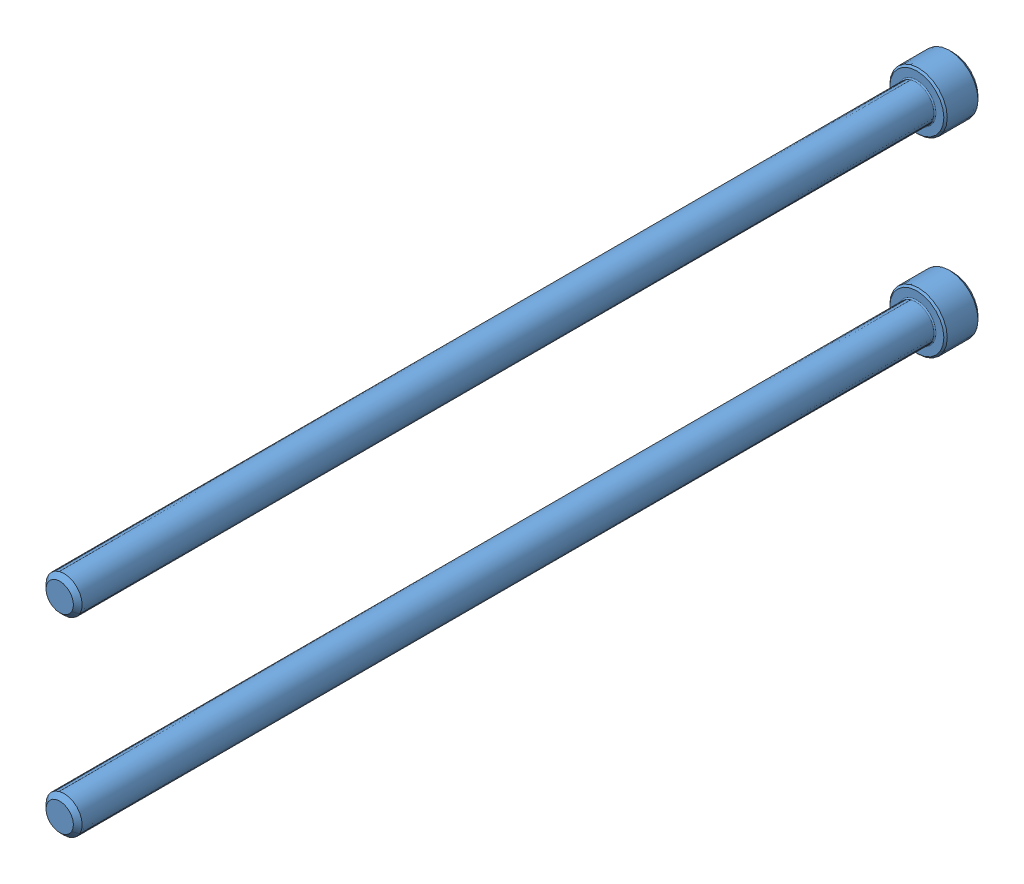
SolidWorks assembly WCP - GreyT Elevator (Cascade, 2 Stage) (1).step, configuration Default. Lengths in mm.
Overall size (10.46 35.86 119.13).
407 component instances, 66 part files, 0 mates.
Components (placement in the parent):
- WCP-0323 - Elevator Clamping Block.step-1: WCP-0323 - Elevator Clamping Block.step [Default] at (152.3365 1149.35 -25.4) x (0 0 1) z (-1 0 0) size (29.22 25.41 49.35) (hidden)
  - WCP-0323-001 Rev2.step-1: WCP-0323-001 Rev2.step [Default] at origin size (20.38 25.41 40.49)
  - WCP-0498 Rev1.step-1: WCP-0498 Rev1.step [Default] at (2.254 0 6.7) x (0 0.307359 0.951594) z (-1 0 0) size (12 12 4)
  - WCP-0212_0_250_radial_bearing.step-1: WCP-0212_0_250_radial_bearing.step [Default] at (-9.525 0 15.4781) size (19.05 19.05 7.14)
  - WCP-0473 Rev1.step-1: WCP-0473 Rev1.step [Default] at (-9.525 0 10.4394) x (-0.082744 -0.996571 0) z (-0.996571 0.082744 0) size (9.53 20.65 9.53)
  - #8-32 x .25L BHCS.step-1: #8-32 x .25L BHCS.step [Default] at (6.7178 0 6.7) x (0 -0.337236 -0.94142) z (1 0 0) size (10.28 8 12.02)
- WCP-0323 - Elevator Clamping Block-1.step-1: WCP-0323 - Elevator Clamping Block-1.step [Default] at (152.3365 1149.35 25.4) x (0 0 -1) z (-1 0 0) size (29.22 25.41 49.35) (hidden)
  - WCP-0323-001 Rev2.step-1: WCP-0323-001 Rev2.step [Default] at origin size (20.38 25.41 40.49)
  - WCP-0498 Rev1.step-1: WCP-0498 Rev1.step [Default] at (2.254 0 6.7) x (0 0.307359 0.951594) z (-1 0 0) size (12 12 4)
  - WCP-0212_0_250_radial_bearing.step-1: WCP-0212_0_250_radial_bearing.step [Default] at (-9.525 0 15.4781) size (19.05 19.05 7.14)
  - WCP-0473 Rev1.step-1: WCP-0473 Rev1.step [Default] at (-9.525 0 10.4394) x (-0.082744 -0.996571 0) z (-0.996571 0.082744 0) size (9.53 20.65 9.53)
  - #8-32 x .25L BHCS.step-1: #8-32 x .25L BHCS.step [Default] at (6.7178 0 6.7) x (0 -0.337236 -0.94142) z (1 0 0) size (10.28 8 12.02)
- WCP-0323 - Elevator Clamping Block-2.step-1: WCP-0323 - Elevator Clamping Block-2.step [Default] at (139.7635 57.15 25.4) x (0 0 -1) z (1 0 0) size (29.22 25.41 49.35) (hidden)
  - WCP-0323-001 Rev2.step-1: WCP-0323-001 Rev2.step [Default] at origin size (20.38 25.41 40.49)
  - WCP-0498 Rev1.step-1: WCP-0498 Rev1.step [Default] at (2.254 0 6.7) x (0 0.307359 0.951594) z (-1 0 0) size (12 12 4)
  - WCP-0212_0_250_radial_bearing.step-1: WCP-0212_0_250_radial_bearing.step [Default] at (-9.525 0 15.4781) size (19.05 19.05 7.14)
  - WCP-0473 Rev1.step-1: WCP-0473 Rev1.step [Default] at (-9.525 0 10.4394) x (-0.082744 -0.996571 0) z (-0.996571 0.082744 0) size (9.53 20.65 9.53)
  - #8-32 x .25L BHCS.step-1: #8-32 x .25L BHCS.step [Default] at (6.7178 0 6.7) x (0 -0.337236 -0.94142) z (1 0 0) size (10.28 8 12.02)
- WCP-0323 - Elevator Clamping Block-3.step-1: WCP-0323 - Elevator Clamping Block-3.step [Default] at (139.7635 57.15 -25.4) x (0 0 1) z (1 0 0) size (29.22 25.41 49.35) (hidden)
  - WCP-0323-001 Rev2.step-1: WCP-0323-001 Rev2.step [Default] at origin size (20.38 25.41 40.49)
  - WCP-0498 Rev1.step-1: WCP-0498 Rev1.step [Default] at (2.254 0 6.7) x (0 0.307359 0.951594) z (-1 0 0) size (12 12 4)
  - WCP-0212_0_250_radial_bearing.step-1: WCP-0212_0_250_radial_bearing.step [Default] at (-9.525 0 15.4781) size (19.05 19.05 7.14)
  - WCP-0473 Rev1.step-1: WCP-0473 Rev1.step [Default] at (-9.525 0 10.4394) x (-0.082744 -0.996571 0) z (-0.996571 0.082744 0) size (9.53 20.65 9.53)
  - #8-32 x .25L BHCS.step-1: #8-32 x .25L BHCS.step [Default] at (6.7178 0 6.7) x (0 -0.337236 -0.94142) z (1 0 0) size (10.28 8 12.02)
- WCP-0323 - Elevator Clamping Block-4.step-1: WCP-0323 - Elevator Clamping Block-4.step [Default] at (101.6635 82.55 25.4) x (0 0 -1) z (1 0 0) size (29.22 25.41 49.35) (hidden)
  - WCP-0323-001 Rev2.step-1: WCP-0323-001 Rev2.step [Default] at origin size (20.38 25.41 40.49)
  - WCP-0498 Rev1.step-1: WCP-0498 Rev1.step [Default] at (2.254 0 6.7) x (0 0.307359 0.951594) z (-1 0 0) size (12 12 4)
  - WCP-0212_0_250_radial_bearing.step-1: WCP-0212_0_250_radial_bearing.step [Default] at (-9.525 0 15.4781) size (19.05 19.05 7.14)
  - WCP-0473 Rev1.step-1: WCP-0473 Rev1.step [Default] at (-9.525 0 10.4394) x (-0.082744 -0.996571 0) z (-0.996571 0.082744 0) size (9.53 20.65 9.53)
  - #8-32 x .25L BHCS.step-1: #8-32 x .25L BHCS.step [Default] at (6.7178 0 6.7) x (0 -0.337236 -0.94142) z (1 0 0) size (10.28 8 12.02)
- WCP-0323 - Elevator Clamping Block-5.step-1: WCP-0323 - Elevator Clamping Block-5.step [Default] at (101.6635 82.55 -25.4) x (0 0 1) z (1 0 0) size (29.22 25.41 49.35) (hidden)
  - WCP-0323-001 Rev2.step-1: WCP-0323-001 Rev2.step [Default] at origin size (20.38 25.41 40.49)
  - WCP-0498 Rev1.step-1: WCP-0498 Rev1.step [Default] at (2.254 0 6.7) x (0 0.307359 0.951594) z (-1 0 0) size (12 12 4)
  - WCP-0212_0_250_radial_bearing.step-1: WCP-0212_0_250_radial_bearing.step [Default] at (-9.525 0 15.4781) size (19.05 19.05 7.14)
  - WCP-0473 Rev1.step-1: WCP-0473 Rev1.step [Default] at (-9.525 0 10.4394) x (-0.082744 -0.996571 0) z (-0.996571 0.082744 0) size (9.53 20.65 9.53)
  - #8-32 x .25L BHCS.step-1: #8-32 x .25L BHCS.step [Default] at (6.7178 0 6.7) x (0 -0.337236 -0.94142) z (1 0 0) size (10.28 8 12.02)
- WCP-0323 - Elevator Clamping Block-6.step-1: WCP-0323 - Elevator Clamping Block-6.step [Default] at (101.6635 222.25 25.4) x (0 0 -1) z (1 0 0) size (29.22 25.41 49.35) (hidden)
  - WCP-0323-001 Rev2.step-1: WCP-0323-001 Rev2.step [Default] at origin size (20.38 25.41 40.49)
  - WCP-0498 Rev1.step-1: WCP-0498 Rev1.step [Default] at (2.254 0 6.7) x (0 0.307359 0.951594) z (-1 0 0) size (12 12 4)
  - WCP-0212_0_250_radial_bearing.step-1: WCP-0212_0_250_radial_bearing.step [Default] at (-9.525 0 15.4781) size (19.05 19.05 7.14)
  - WCP-0473 Rev1.step-1: WCP-0473 Rev1.step [Default] at (-9.525 0 10.4394) x (-0.082744 -0.996571 0) z (-0.996571 0.082744 0) size (9.53 20.65 9.53)
  - #8-32 x .25L BHCS.step-1: #8-32 x .25L BHCS.step [Default] at (6.7178 0 6.7) x (0 -0.337236 -0.94142) z (1 0 0) size (10.28 8 12.02)
- WCP-0323 - Elevator Clamping Block-7.step-1: WCP-0323 - Elevator Clamping Block-7.step [Default] at (101.6635 222.25 -25.4) x (0 0 1) z (1 0 0) size (29.22 25.41 49.35) (hidden)
  - WCP-0323-001 Rev2.step-1: WCP-0323-001 Rev2.step [Default] at origin size (20.38 25.41 40.49)
  - WCP-0498 Rev1.step-1: WCP-0498 Rev1.step [Default] at (2.254 0 6.7) x (0 0.307359 0.951594) z (-1 0 0) size (12 12 4)
  - WCP-0212_0_250_radial_bearing.step-1: WCP-0212_0_250_radial_bearing.step [Default] at (-9.525 0 15.4781) size (19.05 19.05 7.14)
  - WCP-0473 Rev1.step-1: WCP-0473 Rev1.step [Default] at (-9.525 0 10.4394) x (-0.082744 -0.996571 0) z (-0.996571 0.082744 0) size (9.53 20.65 9.53)
  - #8-32 x .25L BHCS.step-1: #8-32 x .25L BHCS.step [Default] at (6.7178 0 6.7) x (0 -0.337236 -0.94142) z (1 0 0) size (10.28 8 12.02)
- WCP-0248 Rev1 - #35 Chain Turnbuckle.step-1: WCP-0248 Rev1 - #35 Chain Turnbuckle.step [Default] at (88.9 1124.7437 -66.675) x (0 -1 0) z (0 0 1) size (55.56 15.05 15.04) (hidden)
  - WCP-0247-001 Rev1.step-1: WCP-0247-001 Rev1.step [Default] at origin size (30.16 9.53 11)
  - NFS-0040_#10-32_jam_nut_left_hand_99961A520.step-1: NFS-0040_#10-32_jam_nut_left_hand_99961A520.step [Default] at (-16.6687 0 0) x (0 0.5 -0.866025) z (0 0.866025 0.5) size (11.01 3.2 11.02)
  - NFS-0037_#10-32_jam_nut_90480A195.step-1: NFS-0037_#10-32_jam_nut_90480A195.step [Default] at (16.6687 0 0) x (0 0.5 0.866025) z (0 -0.866025 0.5) size (11.01 3.2 11.02)
  - WCP-0248-001 Rev1.step-1: WCP-0248-001 Rev1.step [Default] at (23.8125 0 0) x (0 0 1) z (0 1 0) size (9 25.4 9)
  - WCP-0248-002 Rev1.step-1: WCP-0248-002 Rev1.step [Default] at (-23.8125 0 0) x (0 0 -1) z (0 1 0) size (9 25.4 9)
- WCP-0247 Rev1 - #25 Chain Turnbuckle.step-1: WCP-0247 Rev1 - #25 Chain Turnbuckle.step [Default] at (-47.6339 1117.6 -50.8) x (0 1 0) z (-1 0 0) size (50.8 15.05 15.04) (hidden)
  - WCP-0247-001 Rev1.step-1: WCP-0247-001 Rev1.step [Default] at origin size (30.16 9.53 11)
  - NFS-0040_#10-32_jam_nut_left_hand_99961A520.step-1: NFS-0040_#10-32_jam_nut_left_hand_99961A520.step [Default] at (-16.6687 0 0) x (0 0.5 -0.866025) z (0 0.866025 0.5) size (11.01 3.2 11.02)
  - NFS-0037_#10-32_jam_nut_90480A195.step-1: NFS-0037_#10-32_jam_nut_90480A195.step [Default] at (16.6687 0 0) x (0 0.5 0.866025) z (0 -0.866025 0.5) size (11.01 3.2 11.02)
  - WCP-0247-002 Rev2.step-1: WCP-0247-002 Rev2.step [Default] at (22.225 0 0) x (0 0 1) z (0 1 0) size (9 23.02 5.21)
  - WCP-0247-003 Rev2.step-1: WCP-0247-003 Rev2.step [Default] at (-22.225 0 0) x (0 0 -1) z (0 1 0) size (9 23.02 5.21)
- WCP-0323 - Elevator Clamping Block-8.step-1: WCP-0323 - Elevator Clamping Block-8.step [Default] at (-152.3365 1149.35 25.4) x (0 0 -1) z (1 0 0) size (29.22 25.41 49.35) (hidden)
  - WCP-0323-001 Rev2.step-1: WCP-0323-001 Rev2.step [Default] at origin size (20.38 25.41 40.49)
  - WCP-0498 Rev1.step-1: WCP-0498 Rev1.step [Default] at (2.254 0 6.7) x (0 0.307359 0.951594) z (-1 0 0) size (12 12 4)
  - WCP-0212_0_250_radial_bearing.step-1: WCP-0212_0_250_radial_bearing.step [Default] at (-9.525 0 15.4781) size (19.05 19.05 7.14)
  - WCP-0473 Rev1.step-1: WCP-0473 Rev1.step [Default] at (-9.525 0 10.4394) x (-0.082744 -0.996571 0) z (-0.996571 0.082744 0) size (9.53 20.65 9.53)
  - #8-32 x .25L BHCS.step-1: #8-32 x .25L BHCS.step [Default] at (6.7178 0 6.7) x (0 -0.337236 -0.94142) z (1 0 0) size (10.28 8 12.02)
- WCP-0323 - Elevator Clamping Block-9.step-1: WCP-0323 - Elevator Clamping Block-9.step [Default] at (-152.3365 1149.35 -25.4) x (0 0 1) z (1 0 0) size (29.22 25.41 49.35) (hidden)
  - WCP-0323-001 Rev2.step-1: WCP-0323-001 Rev2.step [Default] at origin size (20.38 25.41 40.49)
  - WCP-0498 Rev1.step-1: WCP-0498 Rev1.step [Default] at (2.254 0 6.7) x (0 0.307359 0.951594) z (-1 0 0) size (12 12 4)
  - WCP-0212_0_250_radial_bearing.step-1: WCP-0212_0_250_radial_bearing.step [Default] at (-9.525 0 15.4781) size (19.05 19.05 7.14)
  - WCP-0473 Rev1.step-1: WCP-0473 Rev1.step [Default] at (-9.525 0 10.4394) x (-0.082744 -0.996571 0) z (-0.996571 0.082744 0) size (9.53 20.65 9.53)
  - #8-32 x .25L BHCS.step-1: #8-32 x .25L BHCS.step [Default] at (6.7178 0 6.7) x (0 -0.337236 -0.94142) z (1 0 0) size (10.28 8 12.02)
- WCP-0583 Rev1 - Cascade Pulley Block.step-1: WCP-0583 Rev1 - Cascade Pulley Block.step [Default] at (88.9 25.4 -25.4) x (1 0 0) z (0 1 0) size (47.02 52.05 52.05) (hidden)
  - WCP-0096 Rev6.step-1: WCP-0096 Rev6.step [Default] at (0 25.4 6.35) size (12.65 52.05 52.05)
    - WCP-0096-001 Rev6.step-1: WCP-0096-001 Rev6.step [Default] at origin size (7.57 38.1 38.1)
    - WCP-0096-001 Rev6.step-2: WCP-0096-001 Rev6.step [Default] x (-1 0 0) z (0 0.866025 -0.5) size (7.57 38.1 38.1)
    - WCP-0356 Rev1.step-1: WCP-0356 Rev1.step [Default] at (0.4817 -4.7625 -8.2489) x (0 -0.126969 0.991907) z (0 -0.991907 -0.126969) size (4.06 11.05 4.06)
    - WCP-0356 Rev1.step-2: WCP-0356 Rev1.step [Default] at (0.4817 9.525 0) x (0 0.866766 0.498715) z (0 -0.498715 0.866766) size (4.06 11.05 4.06)
    - WCP-0356 Rev1.step-3: WCP-0356 Rev1.step [Default] at (0.4817 -4.7625 8.2489) x (0 -0.994015 -0.109248) z (0 0.109248 -0.994015) size (4.06 11.05 4.06)
    - WCP-0356 Rev1.step-4: WCP-0356 Rev1.step [Default] at (-0.4817 4.7625 -8.2489) x (0 -0.997555 0.069879) z (0 0.069879 0.997555) size (4.06 11.05 4.06)
    - WCP-0356 Rev1.step-5: WCP-0356 Rev1.step [Default] at (-0.4817 4.7625 8.2489) x (0 -0.7202 -0.693767) z (0 -0.693767 0.7202) size (4.06 11.05 4.06)
    - WCP-0356 Rev1.step-6: WCP-0356 Rev1.step [Default] at (-0.4817 -9.525 0) x (0 -0.997555 0.069879) z (0 0.069879 0.997555) size (4.06 11.05 4.06)
  - WCP-0583-001 Rev1.step-1: WCP-0583-001 Rev1.step [Default] at origin size (34.92 31.75 25.4)
  - WCP-0567 Rev1.step-1: WCP-0567 Rev1.step [Default] at (-6.3246 25.4 6.35) x (0 0 1) z (-1 0 0) size (15.88 15.88 7.94)
  - WCP-0567 Rev1.step-2: WCP-0567 Rev1.step [Default] at (6.3246 25.4 6.35) x (0 0 1) z (1 0 0) size (15.88 15.88 7.94)
  - WCP-0203 Rev1.step-1: WCP-0203 Rev1.step [Default] at (0 25.4 6.35) size (15.88 9.5 9.5)
  - 10-32 BHCS - No Thread_WCP-0258 - 1.750.step-1: 10-32 BHCS - No Thread_WCP-0258 - 1.750.step [Default] at (-17.4625 25.4 6.35) x (0 -0.816967 0.576685) z (0 -0.576685 -0.816967) size (9.17 47.02 9.17)
  - WCP-0326 Rev1.step-1: WCP-0326 Rev1.step [Default] at (19.8374 25.4 6.35) x (0 0.003214 -0.999995) z (0 -0.999995 -0.003214) size (11.02 4.76 11)
- WCP-0583 Rev1 - Cascade Pulley Block-1.step-1: WCP-0583 Rev1 - Cascade Pulley Block-1.step [Default] at (88.9 1219.2 -25.4) x (1 0 0) z (0 1 0) size (47.02 52.05 52.05) (hidden)
  - WCP-0096 Rev6-1.step-1: WCP-0096 Rev6-1.step [Default] at (0 25.4 6.35) size (12.65 52.05 52.05)
    - WCP-0096-001 Rev6.step-1: WCP-0096-001 Rev6.step [Default] at origin size (7.57 38.1 38.1)
    - WCP-0096-001 Rev6.step-2: WCP-0096-001 Rev6.step [Default] x (-1 0 0) z (0 0.866025 -0.5) size (7.57 38.1 38.1)
    - WCP-0356 Rev1.step-1: WCP-0356 Rev1.step [Default] at (0.4817 -4.7625 -8.2489) x (0 -0.126969 0.991907) z (0 -0.991907 -0.126969) size (4.06 11.05 4.06)
    - WCP-0356 Rev1.step-2: WCP-0356 Rev1.step [Default] at (0.4817 9.525 0) x (0 0.866766 0.498715) z (0 -0.498715 0.866766) size (4.06 11.05 4.06)
    - WCP-0356 Rev1.step-3: WCP-0356 Rev1.step [Default] at (0.4817 -4.7625 8.2489) x (0 -0.994015 -0.109248) z (0 0.109248 -0.994015) size (4.06 11.05 4.06)
    - WCP-0356 Rev1.step-4: WCP-0356 Rev1.step [Default] at (-0.4817 4.7625 -8.2489) x (0 -0.997555 0.069879) z (0 0.069879 0.997555) size (4.06 11.05 4.06)
    - WCP-0356 Rev1.step-5: WCP-0356 Rev1.step [Default] at (-0.4817 4.7625 8.2489) x (0 -0.7202 -0.693767) z (0 -0.693767 0.7202) size (4.06 11.05 4.06)
    - WCP-0356 Rev1.step-6: WCP-0356 Rev1.step [Default] at (-0.4817 -9.525 0) x (0 -0.997555 0.069879) z (0 0.069879 0.997555) size (4.06 11.05 4.06)
  - WCP-0583-001 Rev1.step-1: WCP-0583-001 Rev1.step [Default] at origin size (34.92 31.75 25.4)
  - WCP-0567 Rev1.step-1: WCP-0567 Rev1.step [Default] at (-6.3246 25.4 6.35) x (0 0 1) z (-1 0 0) size (15.88 15.88 7.94)
  - WCP-0567 Rev1.step-2: WCP-0567 Rev1.step [Default] at (6.3246 25.4 6.35) x (0 0 1) z (1 0 0) size (15.88 15.88 7.94)
  - WCP-0203 Rev1.step-1: WCP-0203 Rev1.step [Default] at (0 25.4 6.35) size (15.88 9.5 9.5)
  - 10-32 BHCS - No Thread_WCP-0258 - 1.750.step-1: 10-32 BHCS - No Thread_WCP-0258 - 1.750.step [Default] at (-17.4625 25.4 6.35) x (0 -0.816967 0.576685) z (0 -0.576685 -0.816967) size (9.17 47.02 9.17)
  - WCP-0326 Rev1.step-1: WCP-0326 Rev1.step [Default] at (19.8374 25.4 6.35) x (0 0.003214 -0.999995) z (0 -0.999995 -0.003214) size (11.02 4.76 11)
- WCP-0583 Rev1 - Cascade Pulley Block_Mirrored.step-1: WCP-0583 Rev1 - Cascade Pulley Block_Mirrored.step [Default] at (-88.9 1219.2 -25.4) x (1 0 0) z (0 1 0) size (47.02 52.05 52.05) (hidden)
  - WCP-0096 Rev6-2.step-1: WCP-0096 Rev6-2.step [Default] at (0 25.4 6.35) size (12.65 52.05 52.05)
    - WCP-0096-001 Rev6.step-1: WCP-0096-001 Rev6.step [Default] at origin size (7.57 38.1 38.1)
    - WCP-0096-001 Rev6.step-2: WCP-0096-001 Rev6.step [Default] x (-1 0 0) z (0 0.866025 -0.5) size (7.57 38.1 38.1)
    - WCP-0356 Rev1.step-1: WCP-0356 Rev1.step [Default] at (0.4817 -4.7625 -8.2489) x (0 -0.126969 0.991907) z (0 -0.991907 -0.126969) size (4.06 11.05 4.06)
    - WCP-0356 Rev1.step-2: WCP-0356 Rev1.step [Default] at (0.4817 9.525 0) x (0 0.866766 0.498715) z (0 -0.498715 0.866766) size (4.06 11.05 4.06)
    - WCP-0356 Rev1.step-3: WCP-0356 Rev1.step [Default] at (0.4817 -4.7625 8.2489) x (0 -0.994015 -0.109248) z (0 0.109248 -0.994015) size (4.06 11.05 4.06)
    - WCP-0356 Rev1.step-4: WCP-0356 Rev1.step [Default] at (-0.4817 4.7625 -8.2489) x (0 -0.997555 0.069879) z (0 0.069879 0.997555) size (4.06 11.05 4.06)
    - WCP-0356 Rev1.step-5: WCP-0356 Rev1.step [Default] at (-0.4817 4.7625 8.2489) x (0 -0.7202 -0.693767) z (0 -0.693767 0.7202) size (4.06 11.05 4.06)
    - WCP-0356 Rev1.step-6: WCP-0356 Rev1.step [Default] at (-0.4817 -9.525 0) x (0 -0.997555 0.069879) z (0 0.069879 0.997555) size (4.06 11.05 4.06)
  - WCP-0583-001 Rev1.step-1: WCP-0583-001 Rev1.step [Default] at origin size (34.92 31.75 25.4)
  - WCP-0567 Rev1.step-1: WCP-0567 Rev1.step [Default] at (-6.3246 25.4 6.35) x (0 0 1) z (-1 0 0) size (15.88 15.88 7.94)
  - WCP-0567 Rev1.step-2: WCP-0567 Rev1.step [Default] at (6.3246 25.4 6.35) x (0 0 1) z (1 0 0) size (15.88 15.88 7.94)
  - WCP-0203 Rev1.step-1: WCP-0203 Rev1.step [Default] at (0 25.4 6.35) size (15.88 9.5 9.5)
  - 10-32 BHCS - No Thread_WCP-0258 - 1.750.step-1: 10-32 BHCS - No Thread_WCP-0258 - 1.750.step [Default] at (17.4625 25.4 6.35) x (0 0.844944 -0.534854) z (0 -0.534854 -0.844944) size (9.17 47.02 9.17)
  - WCP-0326 Rev1.step-1: WCP-0326 Rev1.step [Default] at (-19.8374 25.4 6.35) x (0 -0.925447 -0.378877) z (0 0.378877 -0.925447) size (11.02 4.76 11)
- WCP-0583 Rev1 - Cascade Pulley Block_Mirrored-1.step-1: WCP-0583 Rev1 - Cascade Pulley Block_Mirrored-1.step [Default] at (-88.9 25.4 -25.4) x (1 0 0) z (0 1 0) size (47.02 52.05 52.05) (hidden)
  - WCP-0096 Rev6-3.step-1: WCP-0096 Rev6-3.step [Default] at (0 25.4 6.35) size (12.65 52.05 52.05)
    - WCP-0096-001 Rev6.step-1: WCP-0096-001 Rev6.step [Default] at origin size (7.57 38.1 38.1)
    - WCP-0096-001 Rev6.step-2: WCP-0096-001 Rev6.step [Default] x (-1 0 0) z (0 0.866025 -0.5) size (7.57 38.1 38.1)
    - WCP-0356 Rev1.step-1: WCP-0356 Rev1.step [Default] at (0.4817 -4.7625 -8.2489) x (0 -0.126969 0.991907) z (0 -0.991907 -0.126969) size (4.06 11.05 4.06)
    - WCP-0356 Rev1.step-2: WCP-0356 Rev1.step [Default] at (0.4817 9.525 0) x (0 0.866766 0.498715) z (0 -0.498715 0.866766) size (4.06 11.05 4.06)
    - WCP-0356 Rev1.step-3: WCP-0356 Rev1.step [Default] at (0.4817 -4.7625 8.2489) x (0 -0.994015 -0.109248) z (0 0.109248 -0.994015) size (4.06 11.05 4.06)
    - WCP-0356 Rev1.step-4: WCP-0356 Rev1.step [Default] at (-0.4817 4.7625 -8.2489) x (0 -0.997555 0.069879) z (0 0.069879 0.997555) size (4.06 11.05 4.06)
    - WCP-0356 Rev1.step-5: WCP-0356 Rev1.step [Default] at (-0.4817 4.7625 8.2489) x (0 -0.7202 -0.693767) z (0 -0.693767 0.7202) size (4.06 11.05 4.06)
    - WCP-0356 Rev1.step-6: WCP-0356 Rev1.step [Default] at (-0.4817 -9.525 0) x (0 -0.997555 0.069879) z (0 0.069879 0.997555) size (4.06 11.05 4.06)
  - WCP-0583-001 Rev1.step-1: WCP-0583-001 Rev1.step [Default] at origin size (34.92 31.75 25.4)
  - WCP-0567 Rev1.step-1: WCP-0567 Rev1.step [Default] at (-6.3246 25.4 6.35) x (0 0 1) z (-1 0 0) size (15.88 15.88 7.94)
  - WCP-0567 Rev1.step-2: WCP-0567 Rev1.step [Default] at (6.3246 25.4 6.35) x (0 0 1) z (1 0 0) size (15.88 15.88 7.94)
  - WCP-0203 Rev1.step-1: WCP-0203 Rev1.step [Default] at (0 25.4 6.35) size (15.88 9.5 9.5)
  - 10-32 BHCS - No Thread_WCP-0258 - 1.750.step-1: 10-32 BHCS - No Thread_WCP-0258 - 1.750.step [Default] at (17.4625 25.4 6.35) x (0 0.844944 -0.534854) z (0 -0.534854 -0.844944) size (9.17 47.02 9.17)
  - WCP-0326 Rev1.step-1: WCP-0326 Rev1.step [Default] at (-19.8374 25.4 6.35) x (0 -0.925447 -0.378877) z (0 0.378877 -0.925447) size (11.02 4.76 11)
- WCP-0323 - Elevator Clamping Block-10.step-1: WCP-0323 - Elevator Clamping Block-10.step [Default] at (-139.7635 57.15 -25.4) x (0 0 1) z (-1 0 0) size (29.22 25.41 49.35) (hidden)
  - WCP-0323-001 Rev2.step-1: WCP-0323-001 Rev2.step [Default] at origin size (20.38 25.41 40.49)
  - WCP-0498 Rev1.step-1: WCP-0498 Rev1.step [Default] at (2.254 0 6.7) x (0 0.307359 0.951594) z (-1 0 0) size (12 12 4)
  - WCP-0212_0_250_radial_bearing.step-1: WCP-0212_0_250_radial_bearing.step [Default] at (-9.525 0 15.4781) size (19.05 19.05 7.14)
  - WCP-0473 Rev1.step-1: WCP-0473 Rev1.step [Default] at (-9.525 0 10.4394) x (-0.082744 -0.996571 0) z (-0.996571 0.082744 0) size (9.53 20.65 9.53)
  - #8-32 x .25L BHCS.step-1: #8-32 x .25L BHCS.step [Default] at (6.7178 0 6.7) x (0 -0.337236 -0.94142) z (1 0 0) size (10.28 8 12.02)
- WCP-0557 Rev1 - WCP Single Stage Gearbox_0.5_ Hex.step-1: WCP-0557 Rev1 - WCP Single Stage Gearbox_0.5_ Hex.step [Default] at (-25.4 0 66.675) x (-1 0 0) z (0 0 -1) size (173.55 82.41 254.05) (hidden)
  - WCP-0557-001 Rev1.step-1: WCP-0557-001 Rev1.step [Default] at origin size (151.92 76.2 6.35)
  - WCP-0557-002 Rev1.step-1: WCP-0557-002 Rev1.step [Default] at (0 0 34.925) size (76.2 76.2 6.35)
  - 217-6515_Falcon_500_Default_As Machined_.step-1: 217-6515_Falcon_500_Default_As Machined_.step [Default] at (45.7962 0 -29.375) x (0.866025 0.5 0) z (0 0 1) size (60 60 115.81)
  - 217-6515_Falcon_500_Default_As Machined_.step-2: 217-6515_Falcon_500_Default_As Machined_.step [Default] at (-45.7962 0 -29.375) x (0.866025 0.5 0) z (0 0 1) size (60 60 115.81)
  - 217-6919_Falcon_12T.step-1: 217-6919_Falcon_12T.step [Default] at (45.7962 0 12.5775) x (0.990666 -0.136309 0) z (0 0 1) size (17.78 17.78 19.05)
  - 217-6919_Falcon_12T.step-2: 217-6919_Falcon_12T.step [Default] at (-45.7962 0 12.5775) x (0.990666 -0.136309 0) z (0 0 1) size (17.78 17.78 19.05)
  - WCP-0226 Rev1.step-1: WCP-0226 Rev1.step [Default] at (32.5438 -32.5438 17.4625) x (0 0 -1) z (0.876265 0.481829 0) size (28.57 9.5 9.5)
  - WCP-0226 Rev1.step-2: WCP-0226 Rev1.step [Default] at (32.5438 32.5438 17.4625) x (0 0 -1) z (-0.524135 0.851635 0) size (28.57 9.5 9.5)
  - WCP-0226 Rev1.step-3: WCP-0226 Rev1.step [Default] at (-32.5438 -32.5438 17.4625) x (0 0 -1) z (0.876265 0.481829 0) size (28.57 9.5 9.5)
  - WCP-0226 Rev1.step-4: WCP-0226 Rev1.step [Default] at (-32.5438 32.5438 17.4625) x (0 0 -1) z (0.876265 0.481829 0) size (28.57 9.5 9.5)
  - WCP-0557-004 Rev1.step-1: WCP-0557-004 Rev1.step [Default] at (0 0 0.7937) x (1 0 0) z (0 -1 0) size (45 7.94 45)
  - WCP-0781_0_500_flanged_bearing.step-1: WCP-0781_0_500_flanged_bearing.step [Default] at (0 0 -3.175) x (0.999832 0.018325 0) z (0.018325 -0.999832 0) size (31.12 7.94 31.12)
  - WCP-0557-004 Rev1.step-2: WCP-0557-004 Rev1.step [Default] at (0 0 34.1313) x (1 0 0) z (0 1 0) size (45 7.94 45)
  - WCP-0790_500L_500_hex.step-1: WCP-0790_500L_500_hex.step [Default] at (0 0 23.7617) x (0.953738 0.300639 0) z (0 0 1) size (19.5 19.5 12.7)
  - 10-32 BHCS - No Thread_WCP-0257 - 1.500.step-1: 10-32 BHCS - No Thread_WCP-0257 - 1.500.step [Default] at (32.5438 32.5438 0) x (0.63562 -0.772002 0) z (0.772002 0.63562 0) size (9.17 40.67 9.17)
  - 10-32 BHCS - No Thread_WCP-0257 - 1.500.step-2: 10-32 BHCS - No Thread_WCP-0257 - 1.500.step [Default] at (-32.5438 32.5438 0) x (0.63562 -0.772002 0) z (0.772002 0.63562 0) size (9.17 40.67 9.17)
  - 10-32 BHCS - No Thread_WCP-0257 - 1.500.step-3: 10-32 BHCS - No Thread_WCP-0257 - 1.500.step [Default] at (32.5438 -32.5438 0) x (0.63562 -0.772002 0) z (0.772002 0.63562 0) size (9.17 40.67 9.17)
  - 10-32 BHCS - No Thread_WCP-0257 - 1.500.step-4: 10-32 BHCS - No Thread_WCP-0257 - 1.500.step [Default] at (-32.5438 -32.5438 0) x (0.63562 -0.772002 0) z (0.772002 0.63562 0) size (9.17 40.67 9.17)
  - 10-32 BHCS - No Thread_WCP-0253 - 0.500.step-1: 10-32 BHCS - No Thread_WCP-0253 - 0.500.step [Default] at (45.7962 25.4 3.175) x (0.313732 -0.949511 0) z (-0.949511 -0.313732 0) size (9.17 15.27 9.17)
  - 10-32 BHCS - No Thread_WCP-0253 - 0.500.step-2: 10-32 BHCS - No Thread_WCP-0253 - 0.500.step [Default] at (45.7962 -25.4 3.175) x (0.270491 -0.962723 0) z (-0.962723 -0.270491 0) size (9.17 15.27 9.17)
  - 10-32 BHCS - No Thread_WCP-0253 - 0.500.step-3: 10-32 BHCS - No Thread_WCP-0253 - 0.500.step [Default] at (-45.7962 25.4 3.175) x (0.363225 -0.931702 0) z (-0.931702 -0.363225 0) size (9.17 15.27 9.17)
  - 10-32 BHCS - No Thread_WCP-0253 - 0.500.step-4: 10-32 BHCS - No Thread_WCP-0253 - 0.500.step [Default] at (-45.7962 -25.4 3.175) x (0.510832 -0.85968 0) z (-0.85968 -0.510832 0) size (9.17 15.27 9.17)
  - WCP-0832 Rev1.step-1: WCP-0832 Rev1.step [Default] at (0 0 87.3125) x (0.457904 0.889002 0) z (0 0 1) size (13.75 13.61 175.64)
  - WCP-0785_0_500_flanged_thunderhex_bearing.step-1: WCP-0785_0_500_flanged_thunderhex_bearing.step [Default] at (0 0 34.1313) x (-0.110978 -0.993823 0) z (0 0 -1) size (31.12 31.12 7.94)
  - WCP-0229 Rev1.step-1: WCP-0229 Rev1.step [Default] at (0 0 -3.6195) x (0 0 1) z (-0.791548 -0.611107 0) size (0.89 16.1 14.34)
  - WCP-0187 Rev1.step-1: WCP-0187 Rev1.step [Default] at (0 0 11.0871) x (0.99882 0.048566 0) z (0 0 1) size (78.68 78.68 12.65)
- WCP-0323 - Elevator Clamping Block-11.step-1: WCP-0323 - Elevator Clamping Block-11.step [Default] at (-101.6635 82.55 -25.4) x (0 0 1) z (-1 0 0) size (29.22 25.41 49.35) (hidden)
  - WCP-0323-001 Rev2.step-1: WCP-0323-001 Rev2.step [Default] at origin size (20.38 25.41 40.49)
  - WCP-0498 Rev1.step-1: WCP-0498 Rev1.step [Default] at (2.254 0 6.7) x (0 0.307359 0.951594) z (-1 0 0) size (12 12 4)
  - WCP-0212_0_250_radial_bearing.step-1: WCP-0212_0_250_radial_bearing.step [Default] at (-9.525 0 15.4781) size (19.05 19.05 7.14)
  - WCP-0473 Rev1.step-1: WCP-0473 Rev1.step [Default] at (-9.525 0 10.4394) x (-0.082744 -0.996571 0) z (-0.996571 0.082744 0) size (9.53 20.65 9.53)
  - #8-32 x .25L BHCS.step-1: #8-32 x .25L BHCS.step [Default] at (6.7178 0 6.7) x (0 -0.337236 -0.94142) z (1 0 0) size (10.28 8 12.02)
- WCP-0323 - Elevator Clamping Block-12.step-1: WCP-0323 - Elevator Clamping Block-12.step [Default] at (-101.6635 82.55 25.4) x (0 0 -1) z (-1 0 0) size (29.22 25.41 49.35) (hidden)
  - WCP-0323-001 Rev2.step-1: WCP-0323-001 Rev2.step [Default] at origin size (20.38 25.41 40.49)
  - WCP-0498 Rev1.step-1: WCP-0498 Rev1.step [Default] at (2.254 0 6.7) x (0 0.307359 0.951594) z (-1 0 0) size (12 12 4)
  - WCP-0212_0_250_radial_bearing.step-1: WCP-0212_0_250_radial_bearing.step [Default] at (-9.525 0 15.4781) size (19.05 19.05 7.14)
  - WCP-0473 Rev1.step-1: WCP-0473 Rev1.step [Default] at (-9.525 0 10.4394) x (-0.082744 -0.996571 0) z (-0.996571 0.082744 0) size (9.53 20.65 9.53)
  - #8-32 x .25L BHCS.step-1: #8-32 x .25L BHCS.step [Default] at (6.7178 0 6.7) x (0 -0.337236 -0.94142) z (1 0 0) size (10.28 8 12.02)
- WCP-0323 - Elevator Clamping Block-13.step-1: WCP-0323 - Elevator Clamping Block-13.step [Default] at (-139.7635 57.15 25.4) x (0 0 -1) z (-1 0 0) size (29.22 25.41 49.35) (hidden)
  - WCP-0323-001 Rev2.step-1: WCP-0323-001 Rev2.step [Default] at origin size (20.38 25.41 40.49)
  - WCP-0498 Rev1.step-1: WCP-0498 Rev1.step [Default] at (2.254 0 6.7) x (0 0.307359 0.951594) z (-1 0 0) size (12 12 4)
  - WCP-0212_0_250_radial_bearing.step-1: WCP-0212_0_250_radial_bearing.step [Default] at (-9.525 0 15.4781) size (19.05 19.05 7.14)
  - WCP-0473 Rev1.step-1: WCP-0473 Rev1.step [Default] at (-9.525 0 10.4394) x (-0.082744 -0.996571 0) z (-0.996571 0.082744 0) size (9.53 20.65 9.53)
  - #8-32 x .25L BHCS.step-1: #8-32 x .25L BHCS.step [Default] at (6.7178 0 6.7) x (0 -0.337236 -0.94142) z (1 0 0) size (10.28 8 12.02)
- WCP-0323 - Elevator Clamping Block-14.step-1: WCP-0323 - Elevator Clamping Block-14.step [Default] at (-101.6635 222.25 -25.4) x (0 0 1) z (-1 0 0) size (29.22 25.41 49.35) (hidden)
  - WCP-0323-001 Rev2.step-1: WCP-0323-001 Rev2.step [Default] at origin size (20.38 25.41 40.49)
  - WCP-0498 Rev1.step-1: WCP-0498 Rev1.step [Default] at (2.254 0 6.7) x (0 0.307359 0.951594) z (-1 0 0) size (12 12 4)
  - WCP-0212_0_250_radial_bearing.step-1: WCP-0212_0_250_radial_bearing.step [Default] at (-9.525 0 15.4781) size (19.05 19.05 7.14)
  - WCP-0473 Rev1.step-1: WCP-0473 Rev1.step [Default] at (-9.525 0 10.4394) x (-0.082744 -0.996571 0) z (-0.996571 0.082744 0) size (9.53 20.65 9.53)
  - #8-32 x .25L BHCS.step-1: #8-32 x .25L BHCS.step [Default] at (6.7178 0 6.7) x (0 -0.337236 -0.94142) z (1 0 0) size (10.28 8 12.02)
- WCP-0323 - Elevator Clamping Block-15.step-1: WCP-0323 - Elevator Clamping Block-15.step [Default] at (-101.6635 222.25 25.4) x (0 0 -1) z (-1 0 0) size (29.22 25.41 49.35) (hidden)
  - WCP-0323-001 Rev2.step-1: WCP-0323-001 Rev2.step [Default] at origin size (20.38 25.41 40.49)
  - WCP-0498 Rev1.step-1: WCP-0498 Rev1.step [Default] at (2.254 0 6.7) x (0 0.307359 0.951594) z (-1 0 0) size (12 12 4)
  - WCP-0212_0_250_radial_bearing.step-1: WCP-0212_0_250_radial_bearing.step [Default] at (-9.525 0 15.4781) size (19.05 19.05 7.14)
  - WCP-0473 Rev1.step-1: WCP-0473 Rev1.step [Default] at (-9.525 0 10.4394) x (-0.082744 -0.996571 0) z (-0.996571 0.082744 0) size (9.53 20.65 9.53)
  - #8-32 x .25L BHCS.step-1: #8-32 x .25L BHCS.step [Default] at (6.7178 0 6.7) x (0 -0.337236 -0.94142) z (1 0 0) size (10.28 8 12.02)
- WCP-0248 Rev1 - #35 Chain Turnbuckle-1.step-1: WCP-0248 Rev1 - #35 Chain Turnbuckle-1.step [Default] at (-88.9 1124.7437 -66.675) x (0 -1 0) z (0 0 -1) size (55.56 15.05 15.04) (hidden)
  - WCP-0247-001 Rev1.step-1: WCP-0247-001 Rev1.step [Default] at origin size (30.16 9.53 11)
  - NFS-0040_#10-32_jam_nut_left_hand_99961A520.step-1: NFS-0040_#10-32_jam_nut_left_hand_99961A520.step [Default] at (-16.6687 0 0) x (0 0.5 -0.866025) z (0 0.866025 0.5) size (11.01 3.2 11.02)
  - NFS-0037_#10-32_jam_nut_90480A195.step-1: NFS-0037_#10-32_jam_nut_90480A195.step [Default] at (16.6687 0 0) x (0 0.5 0.866025) z (0 -0.866025 0.5) size (11.01 3.2 11.02)
  - WCP-0248-001 Rev1.step-1: WCP-0248-001 Rev1.step [Default] at (23.8125 0 0) x (0 0 1) z (0 1 0) size (9 25.4 9)
  - WCP-0248-002 Rev1.step-1: WCP-0248-002 Rev1.step [Default] at (-23.8125 0 0) x (0 0 -1) z (0 1 0) size (9 25.4 9)
- WCP-EX-0019-001.step-1: WCP-EX-0019-001.step [Default] x (1 0 0) z (0 -1 0) size (457.2 50.8 25.4) (hidden)
- WCP-EX-0019-003.step-1: WCP-EX-0019-003.step [Default] at (165.1 609.6 0) x (0 -1 0) z (1 0 0) size (1193.8 50.8 25.4) (hidden)
- WCP-EX-0019-002.step-1: WCP-EX-0019-002.step [Default] at (0 1181.1 -88.9) size (355.6 50.8 25.4) (hidden)
- WCP-EX-0019-004.step-1: WCP-EX-0019-004.step [Default] at (127 622.3 0) x (0 -1 0) z (-1 0 0) size (1219.2 50.8 25.4) (hidden)
- WCP-EX-0019-007.step-1: WCP-EX-0019-007.step [Default] at (0 25.4 0) x (1 0 0) z (0 -1 0) size (228.6 50.8 25.4) (hidden)
- WCP-EX-0019-007.step-2: WCP-EX-0019-007.step [Default] at (0 1219.2 0) x (1 0 0) z (0 -1 0) size (228.6 50.8 25.4) (hidden)
- WCP-EX-0019-005.step-1: WCP-EX-0019-005.step [Default] at (88.9 152.4 0) x (0 -1 0) z (-1 0 0) size (228.6 50.8 25.4) (hidden)
- WCP-EX-0019-006.step-1: WCP-EX-0019-006.step [Default] at (0 50.8 0) x (1 0 0) z (0 -1 0) size (152.4 50.8 25.4) (hidden)
- WCP-EX-0019-006.step-2: WCP-EX-0019-006.step [Default] at (0 254 0) x (1 0 0) z (0 -1 0) size (152.4 50.8 25.4) (hidden)
- WCP-EX-0019-003.step-2: WCP-EX-0019-003.step [Default] at (-165.1 609.6 0) x (0 -1 0) z (1 0 0) size (1193.8 50.8 25.4) (hidden)
- 10-32 BHCS - No Thread_WCP-0261 - 2.500.step-1: 10-32 BHCS - No Thread_WCP-0261 - 2.500.step [Default] at (165.1 1143 30.1625) x (0.999937 0.011255 0) z (0.011255 -0.999937 0) size (9.17 66.07 9.17) (hidden)
- 10-32 BHCS - No Thread_WCP-0261 - 2.500.step-2: 10-32 BHCS - No Thread_WCP-0261 - 2.500.step [Default] at (165.1 1155.7 -30.1625) x (-0.802481 0.596678 0) z (-0.596678 -0.802481 0) size (9.17 66.07 9.17) (hidden)
- 10-32 BHCS - No Thread_WCP-0261 - 2.500.step-3: 10-32 BHCS - No Thread_WCP-0261 - 2.500.step [Default] at (127 50.8 -30.1625) x (-0.742242 0.670132 0) z (-0.670132 -0.742242 0) size (9.17 66.07 9.17) (hidden)
- 10-32 BHCS - No Thread_WCP-0261 - 2.500.step-4: 10-32 BHCS - No Thread_WCP-0261 - 2.500.step [Default] at (127 63.5 30.1625) x (0.985295 -0.170861 0) z (-0.170861 -0.985295 0) size (9.17 66.07 9.17) (hidden)
- 10-32 BHCS - No Thread_WCP-0261 - 2.500.step-5: 10-32 BHCS - No Thread_WCP-0261 - 2.500.step [Default] at (88.9 76.2 -30.1625) x (-0.742242 0.670132 0) z (-0.670132 -0.742242 0) size (9.17 66.07 9.17) (hidden)
- 10-32 BHCS - No Thread_WCP-0261 - 2.500.step-6: 10-32 BHCS - No Thread_WCP-0261 - 2.500.step [Default] at (88.9 88.9 30.1625) x (0.985295 -0.170861 0) z (-0.170861 -0.985295 0) size (9.17 66.07 9.17) (hidden)
- 10-32 BHCS - No Thread_WCP-0261 - 2.500.step-7: 10-32 BHCS - No Thread_WCP-0261 - 2.500.step [Default] at (88.9 215.9 -30.1625) x (-0.742242 0.670132 0) z (-0.670132 -0.742242 0) size (9.17 66.07 9.17) (hidden)
- 10-32 BHCS - No Thread_WCP-0261 - 2.500.step-8: 10-32 BHCS - No Thread_WCP-0261 - 2.500.step [Default] at (88.9 228.6 30.1625) x (0.985295 -0.170861 0) z (-0.170861 -0.985295 0) size (9.17 66.07 9.17) (hidden)
- 10-32 SHCS - No Thread_WCP-0274 - 4.500.step-1: 10-32 SHCS - No Thread_WCP-0274 - 4.500.step [Default] at (165.1 1168.4 -77.7875) x (0.495006 -0.86889 0) z (0.86889 0.495006 0) size (7.67 119.13 7.67) (hidden)
